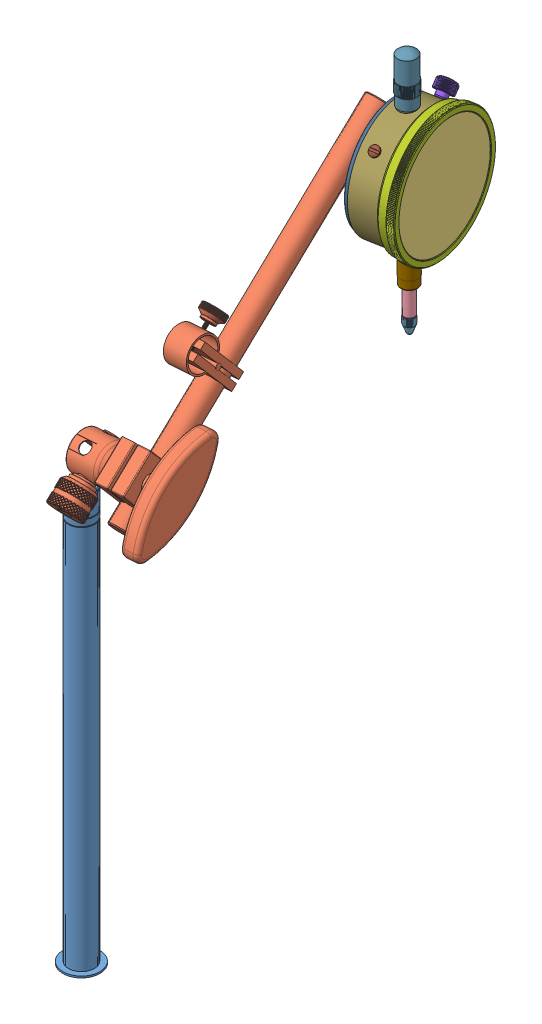
SolidWorks assembly dial high, configuration Default. Lengths in mm.
Overall size (67.74 325.5 171.48).
18 component instances, 14 part files, 0 mates.
Components (placement in the parent):
- rod-1: rod [2310A15] at origin size (17 191.26 17)
- arm-1: arm [2310A15] at (26.9428 323.3212 -156.3074) x (0.997726 0.067336 0.003074) z (0.053395 -0.761691 -0.645736) size (45.9 172.8 31.52)
- Dial indicator - Mitutoyo NO.2046.step-1: Dial indicator - Mitutoyo NO.2046.step [Default] at (30.1473 304.3211 -113.969) x (-0.165048 0 -0.986286) z (-0.008607 0.999962 0.00144) size (57.45 42.2 113.3)
  - Glass.step-1: Glass.step [Default] at (0 -18.65 0) x (0 0 1) z (-1 0 0) size (51.5 1.75 51.5)
  - Shaft.step-1: Shaft.step [Default] at (0 -5.75 29) size (6 6 90.9)
  - Tip.step-1: Tip.step [Default] at (0 -5.75 -52.3) size (5 5 12.5)
  - Back screw.step-1: Back screw.step [Default] at (16.2988 -3.2 -16.2988) x (0.707107 0 0.707107) z (0 1 0) size (3 3 5)
  - Dial.step-1: Dial.step [Default] at (0 -15.1 0) size (57.45 8.05 57.45)
  - Back screw.step-2: Back screw.step [Default] at (-16.2988 -3.2 -16.2988) x (0.707107 0 -0.707107) z (0 1 0) size (3 3 5)
  - Back screw.step-3: Back screw.step [Default] at (-16.2988 -3.2 16.2988) x (0.707107 0 0.707107) z (0 1 0) size (3 3 5)
  - Knurled screw.step-1: Knurled screw.step [Default] at (15.9356 -5.75 15.9356) x (0.707107 0 -0.707107) z (0.707107 0 0.707107) size (8.17 8.17 10.7)
  - Stem.step-1: Stem.step [Default] at (0 -5.85 -45.0423) size (7.9 7.9 24)
  - Back screw.step-4: Back screw.step [Default] at (16.2988 -3.2 16.2988) x (-0.707107 0 0.707107) z (0 1 0) size (3 3 5)
  - Back cover and lug.step-1: Back cover and lug.step [Default] x (1 0 0) z (0 0 -1) size (50.2 21.55 50.2)
  - M2.5x3.7.step-1: M2.5x3.7.step [Default] at (-19.6479 -5.75 19.6479) x (-0.707107 0 -0.707107) z (-0.707107 0 0.707107) size (4.4 4.4 5.4)
  - Case.step-1: Case.step [Default] at origin size (52 15.1 55.04)
  - Long pointer.step-1: Long pointer.step [Default] at (0 -18.6 0) x (0.431825 0 0.901957) z (-0.901957 0 0.431825) size (3.8 6.56 25.9)
  - Cover knob.step-1: Cover knob.step [Default] at (0 -5.75 26.5) size (8.99 8.99 22)
